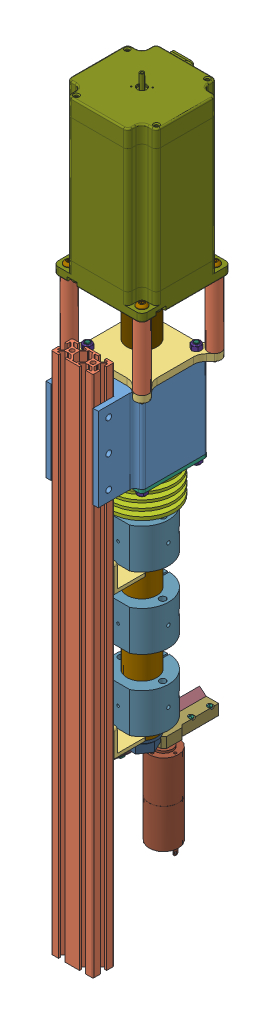
SolidWorks assembly standalone extruder, configuration Default. Lengths in mm.
Overall size (85.21 706.93 142.23).
73 component instances, 27 part files, 167 mates.
Components (placement in the parent):
- hopper rev02-1: hopper rev02 [Default] at (27.6432 17.1739 46.7145) size (63.5 80 98.5)
- 500mm 2040-1: 500mm 2040 [Default] at (27.6432 125.0393 103.4645) x (0 0 1) z (0 1 0) size (20 40 500)
- thrust bearing plate-1: thrust bearing plate [Default] at (27.6432 97.1739 46.7145) size (83.7 6.35 85.2)
- 5909K310_THRUST NEEDLE-ROLLER BEARING-1: 5909K310_THRUST NEEDLE-ROLLER BEARING [5909K31] at (27.6432 95.3689 46.7145) size (23.81 19.84 23.81)
- 5909K440_THRUST NEEDLE-ROLLER BEARING-1: 5909K440_THRUST NEEDLE-ROLLER BEARING [5909K44] at (27.6432 93.5639 46.7145) x (0 1 0) z (0.735724 0 0.677282) size (0.81 23.81 23.81)
- 5909K440_THRUST NEEDLE-ROLLER BEARING-2: 5909K440_THRUST NEEDLE-ROLLER BEARING [5909K44] at (27.6432 96.3611 46.7145) x (0 1 0) z (-0.546944 0 0.837169) size (0.81 23.81 23.81)
- barrel lock mount-1: barrel lock mount [Default] at (27.6432 17.1739 46.7145) x (-1 0 0) z (0 0 1) size (63.5 3.17 63.5)
- barrel lock-1: barrel lock [Default] at (27.6432 -17.7511 46.7145) x (-0.997738 0 -0.067218) z (0.067218 0 -0.997738) size (60.96 31.75 60.96)
- screw standin-1: screw standin [Default] at (27.6432 -173.1361 46.7145) x (0.133635 0 0.991031) z (-0.991031 0 0.133635) size (19.05 324.71 19.05)
- extruder barrel_rev01-1: extruder barrel_rev01 [Default] at (27.6432 93.3739 46.7145) x (1 0 0) z (0 -1 0) size (28.57 28.57 304.8)
- nozzle_rev01-1: nozzle_rev01 [Default] at (27.6432 -192.3761 46.7145) x (0.565776 0 -0.824559) z (0 -1 0) size (28.57 28.57 31.75)
- 3262_1-1: 3262_1 [Default] at (18.029 -323.6244 16.239) x (1 0 0) z (0 1 0) size (28 28 106.2)
- blade wheel-1: blade wheel [Default] at (18.029 -229.4244 16.239) x (0 0 -1) z (-1 0 0) size (90 10 20)
- blade fin-1: blade fin [Default] at (19.9663 -232.1583 46.2387) x (-0.766044 -0.642788 0) z (0 0 -1) size (23.8 0.5 30)
- blade fin-2: blade fin [Default] at (16.0917 -232.1583 -13.7606) x (0.766044 -0.642788 0) z (0 0 1) size (23.8 0.5 30)
- dual cartridge heater block pelletizer-1: dual cartridge heater block pelletizer [Default] at (27.6432 -200.2361 46.7145) x (0 0 1) z (-1 0 0) size (48.25 38.1 50.8)
- dual cartridge heater block pelletizer-2: dual cartridge heater block pelletizer [Default] at (27.6432 -132.1361 46.7145) x (0 0 1) z (-1 0 0) size (48.25 38.1 50.8)
- dual cartridge heater block pelletizer-3: dual cartridge heater block pelletizer [Default] at (27.6432 -64.0361 46.7145) x (0 0 1) z (-1 0 0) size (48.25 38.1 50.8)
- 93325A413_GRADE B7 MEDIUM STRENGTH STEEL THREADED ROD-1: 93325A413_GRADE B7 MEDIUM STRENGTH STEEL THREADED ROD [93325A413] at (53.686 58.9989 20.6718) x (0 -1 0) z (0 0 1) size (101.5 5.07 5.77)
- 93325A413_GRADE B7 MEDIUM STRENGTH STEEL THREADED ROD-2: 93325A413_GRADE B7 MEDIUM STRENGTH STEEL THREADED ROD [93325A413] at (53.686 58.9989 72.7573) x (0 -1 0) z (-0.546944 0 0.837169) size (101.5 5.07 5.77)
- 93325A413_GRADE B7 MEDIUM STRENGTH STEEL THREADED ROD-3: 93325A413_GRADE B7 MEDIUM STRENGTH STEEL THREADED ROD [93325A413] at (1.6005 58.9989 72.7573) x (0 1 0) z (-0.546944 0 0.837169) size (101.5 5.07 5.77)
- 93325A413_GRADE B7 MEDIUM STRENGTH STEEL THREADED ROD-4: 93325A413_GRADE B7 MEDIUM STRENGTH STEEL THREADED ROD [93325A413] at (1.6005 58.9989 20.6718) x (0 -1 0) z (-0.546944 0 0.837169) size (101.5 5.07 5.77)
- nema 34-1: nema 34 [Default] at (27.6432 165.5239 46.7145) x (1 0 0) z (0 -1 0) size (85.21 93.2 198.32)
- 94645A102_ZINC-PLATED CLASS 10 STL NYLON-INSERT LOCKNUT-1: 94645A102_ZINC-PLATED CLASS 10 STL NYLON-INSERT LOCKNUT [94645A102] at (53.686 103.5239 72.7573) size (8 5.15 9.24)
- 94645A102_ZINC-PLATED CLASS 10 STL NYLON-INSERT LOCKNUT-2: 94645A102_ZINC-PLATED CLASS 10 STL NYLON-INSERT LOCKNUT [94645A102] at (53.686 103.5239 20.6718) size (8 5.15 9.24)
- 94645A102_ZINC-PLATED CLASS 10 STL NYLON-INSERT LOCKNUT-3: 94645A102_ZINC-PLATED CLASS 10 STL NYLON-INSERT LOCKNUT [94645A102] at (1.6005 103.5239 72.7573) size (8 5.15 9.24)
- 94645A102_ZINC-PLATED CLASS 10 STL NYLON-INSERT LOCKNUT-4: 94645A102_ZINC-PLATED CLASS 10 STL NYLON-INSERT LOCKNUT [94645A102] at (1.6005 103.5239 20.6718) size (8 5.15 9.24)
- 94645A102_ZINC-PLATED CLASS 10 STL NYLON-INSERT LOCKNUT-5: 94645A102_ZINC-PLATED CLASS 10 STL NYLON-INSERT LOCKNUT [94645A102] at (53.686 13.9989 20.6718) x (-0.5 0 -0.866025) z (-0.866025 0 0.5) size (8 5.15 9.24)
- 94645A102_ZINC-PLATED CLASS 10 STL NYLON-INSERT LOCKNUT-6: 94645A102_ZINC-PLATED CLASS 10 STL NYLON-INSERT LOCKNUT [94645A102] at (53.686 13.9989 72.7573) x (-0.5 0 -0.866025) z (-0.866025 0 0.5) size (8 5.15 9.24)
- 94645A102_ZINC-PLATED CLASS 10 STL NYLON-INSERT LOCKNUT-7: 94645A102_ZINC-PLATED CLASS 10 STL NYLON-INSERT LOCKNUT [94645A102] at (1.6005 13.9989 72.7573) x (-0.5 0 -0.866025) z (-0.866025 0 0.5) size (8 5.15 9.24)
- 94645A102_ZINC-PLATED CLASS 10 STL NYLON-INSERT LOCKNUT-8: 94645A102_ZINC-PLATED CLASS 10 STL NYLON-INSERT LOCKNUT [94645A102] at (1.6005 13.9989 20.6718) x (-0.5 0 -0.866025) z (-0.866025 0 0.5) size (8 5.15 9.24)
- motor coupler-1: motor coupler [Default] at (27.6432 111.6639 46.7145) x (-1 0 0) z (0 0 -1) size (28.57 40 28.57)
- 93245A110_NONMARRING FLAT POINT SOCKET SET SCREW-3: 93245A110_NONMARRING FLAT POINT SOCKET SET SCREW [93245A110] at (27.6432 145.3139 34.7745) x (-0.923728 -0.383049 0) z (0 0 -1) size (4.62 4.16 4.74)
- 93245A110_NONMARRING FLAT POINT SOCKET SET SCREW-4: 93245A110_NONMARRING FLAT POINT SOCKET SET SCREW [93245A110] at (19.2932 118.0139 46.7145) x (0 0.992337 0.12356) z (-1 0 0) size (4.62 4.16 4.74)
- 93245A110_NONMARRING FLAT POINT SOCKET SET SCREW-5: 93245A110_NONMARRING FLAT POINT SOCKET SET SCREW [93245A110] at (27.6432 118.0139 38.3645) x (-0.923728 -0.383049 0) z (0 0 -1) size (4.62 4.16 4.74)
- 93245A110_NONMARRING FLAT POINT SOCKET SET SCREW-6: 93245A110_NONMARRING FLAT POINT SOCKET SET SCREW [93245A110] at (17.7057 145.3139 46.7145) x (0 0.989125 0.14708) z (-1 0 0) size (4.62 4.16 4.74)
- 93245A110_NONMARRING FLAT POINT SOCKET SET SCREW-8: 93245A110_NONMARRING FLAT POINT SOCKET SET SCREW [93245A110] at (28.6332 1.6073 32.0204) x (-0.924173 -0.376865 -0.062262) z (0.067218 0 -0.997738) size (4.62 4.16 4.74)
- motor standoff-1: motor standoff [Default] at (62.3932 103.5239 81.4645) size (12.7 62 12.7)
- motor standoff-2: motor standoff [Default] at (62.3932 103.5239 11.9645) size (12.7 62 12.7)
- motor standoff-3: motor standoff [Default] at (-7.1068 103.5239 81.4645) size (12.7 62 12.7)
- motor standoff-4: motor standoff [Default] at (-7.1068 103.5239 11.9645) size (12.7 62 12.7)
- extruder support-1: extruder support [Default] at (7.6432 -203.4111 93.4645) x (0 -1 0) z (0 0 1) size (25.4 40 31.75)
- extruder support-2: extruder support [Default] at (7.6432 -67.2111 93.4645) x (0 -1 0) z (0 0 1) size (25.4 40 31.75)
- 91239A222_CLASS 10.9 STL BUTTON-HEAD SOCKET CAP SCREW-1: 91239A222_CLASS 10.9 STL BUTTON-HEAD SOCKET CAP SCREW [91239A222] at (17.6432 -206.1611 65.2883) x (1 0 0) z (0 -1 0) size (9.5 9.5 11.19)
- 91239A222_CLASS 10.9 STL BUTTON-HEAD SOCKET CAP SCREW-2: 91239A222_CLASS 10.9 STL BUTTON-HEAD SOCKET CAP SCREW [91239A222] at (37.6432 -206.1611 65.2883) x (1 0 0) z (0 -1 0) size (9.5 9.5 11.19)
- 91239A222_CLASS 10.9 STL BUTTON-HEAD SOCKET CAP SCREW-3: 91239A222_CLASS 10.9 STL BUTTON-HEAD SOCKET CAP SCREW [91239A222] at (37.6432 -69.9611 65.2883) x (1 0 0) z (0 -1 0) size (9.5 9.5 11.19)
- 91239A222_CLASS 10.9 STL BUTTON-HEAD SOCKET CAP SCREW-4: 91239A222_CLASS 10.9 STL BUTTON-HEAD SOCKET CAP SCREW [91239A222] at (17.6432 -69.9611 65.2883) x (1 0 0) z (0 -1 0) size (9.5 9.5 11.19)
- 94180A331_METRIC BRASS HEAT-SET INSERT FOR PLASTICS-1: 94180A331_METRIC BRASS HEAT-SET INSERT FOR PLASTICS [94180A331] at (19.5702 -234.4244 -22.7606) x (-0.492131 0.412947 -0.766344) z (-0.587053 0.492596 0.642431) size (5.56 4.12 5.56)
- 94180A331_METRIC BRASS HEAT-SET INSERT FOR PLASTICS-2: 94180A331_METRIC BRASS HEAT-SET INSERT FOR PLASTICS [94180A331] at (19.5702 -234.4244 -4.7606) x (-0.492131 0.412947 -0.766344) z (-0.587053 0.492596 0.642431) size (5.56 4.12 5.56)
- 94180A331_METRIC BRASS HEAT-SET INSERT FOR PLASTICS-3: 94180A331_METRIC BRASS HEAT-SET INSERT FOR PLASTICS [94180A331] at (16.4877 -234.4244 37.2387) x (-0.613114 -0.514464 -0.599514) z (-0.459255 -0.38536 0.800364) size (5.56 4.12 5.56)
- 94180A331_METRIC BRASS HEAT-SET INSERT FOR PLASTICS-4: 94180A331_METRIC BRASS HEAT-SET INSERT FOR PLASTICS [94180A331] at (16.4877 -234.4244 55.2387) x (-0.613114 -0.514464 -0.599514) z (-0.459255 -0.38536 0.800364) size (5.56 4.12 5.56)
- 92095A181_18-8 SS BUTTON-HEAD SOCKET CAP SCREW-1: 92095A181_18-8 SS BUTTON-HEAD SOCKET CAP SCREW [92095A181] at (17.8697 -236.0714 55.2387) x (0.586824 0.492404 -0.642788) z (0.642788 -0.766044 0) size (5.7 5.7 9.95)
- 92095A181_18-8 SS BUTTON-HEAD SOCKET CAP SCREW-2: 92095A181_18-8 SS BUTTON-HEAD SOCKET CAP SCREW [92095A181] at (17.8697 -236.0714 37.2387) x (0.586824 0.492404 -0.642788) z (0.642788 -0.766044 0) size (5.7 5.7 9.95)
- 92095A181_18-8 SS BUTTON-HEAD SOCKET CAP SCREW-3: 92095A181_18-8 SS BUTTON-HEAD SOCKET CAP SCREW [92095A181] at (18.1882 -236.0714 -4.7606) x (0.586824 -0.492404 0.642788) z (-0.642788 -0.766044 0) size (5.7 5.7 9.95)
- 92095A181_18-8 SS BUTTON-HEAD SOCKET CAP SCREW-4: 92095A181_18-8 SS BUTTON-HEAD SOCKET CAP SCREW [92095A181] at (18.1882 -236.0714 -22.7606) x (0.586824 -0.492404 0.642788) z (-0.642788 -0.766044 0) size (5.7 5.7 9.95)
- 94180A331_METRIC BRASS HEAT-SET INSERT FOR PLASTICS-5: 94180A331_METRIC BRASS HEAT-SET INSERT FOR PLASTICS [94180A331] at (8.029 -234.4244 16.239) x (0 -0.381849 0.924225) z (0 -0.924225 -0.381849) size (5.56 4.12 5.56)
- 92095A181_18-8 SS BUTTON-HEAD SOCKET CAP SCREW-5: 92095A181_18-8 SS BUTTON-HEAD SOCKET CAP SCREW [92095A181] at (5.8682 -234.4244 16.239) x (0 0 1) z (-1 0 0) size (5.7 5.7 9.95)
- 91239A222_CLASS 10.9 STL BUTTON-HEAD SOCKET CAP SCREW-5: 91239A222_CLASS 10.9 STL BUTTON-HEAD SOCKET CAP SCREW [91239A222] at (17.6432 -52.9236 87.5395) x (-0.923728 -0.383049 0) z (0 0 -1) size (9.5 9.5 11.19)
- 91239A222_CLASS 10.9 STL BUTTON-HEAD SOCKET CAP SCREW-6: 91239A222_CLASS 10.9 STL BUTTON-HEAD SOCKET CAP SCREW [91239A222] at (37.6432 -52.9236 87.5395) x (-0.923728 -0.383049 0) z (0 0 -1) size (9.5 9.5 11.19)
- 91239A222_CLASS 10.9 STL BUTTON-HEAD SOCKET CAP SCREW-7: 91239A222_CLASS 10.9 STL BUTTON-HEAD SOCKET CAP SCREW [91239A222] at (37.6432 -189.1236 87.5395) x (-0.923728 -0.383049 0) z (0 0 -1) size (9.5 9.5 11.19)
- 91239A222_CLASS 10.9 STL BUTTON-HEAD SOCKET CAP SCREW-8: 91239A222_CLASS 10.9 STL BUTTON-HEAD SOCKET CAP SCREW [91239A222] at (17.6432 -189.1236 87.5395) x (-0.923728 -0.383049 0) z (0 0 -1) size (9.5 9.5 11.19)
- HNKK5-5-1: HNKK5-5 [Default] at (17.6432 -189.1236 95.4645) x (0 0 -1) z (0 1 0) size (3 10 15)
- HNKK5-5-2: HNKK5-5 [Default] at (37.6432 -189.1236 95.4645) x (0 0 -1) z (0 1 0) size (3 10 15)
- HNKK5-5-3: HNKK5-5 [Default] at (17.6432 -52.9236 95.4645) x (0 0 -1) z (0 1 0) size (3 10 15)
- HNKK5-5-4: HNKK5-5 [Default] at (37.6432 -52.9236 95.4645) x (0 0 -1) z (0 1 0) size (3 10 15)
- 92125A208_TYPE 18-8 SS FLAT-HEAD SOCKET CAP SCREW-1: 92125A208_TYPE 18-8 SS FLAT-HEAD SOCKET CAP SCREW [92125A208] at (13.2748 17.1739 61.0829) x (-0.837169 0 -0.546944) z (0 1 0) size (10 10 10.44)
- 92125A208_TYPE 18-8 SS FLAT-HEAD SOCKET CAP SCREW-2: 92125A208_TYPE 18-8 SS FLAT-HEAD SOCKET CAP SCREW [92125A208] at (13.2748 17.1739 32.3461) x (-0.837169 0 -0.546944) z (0 1 0) size (10 10 10.44)
- 92125A208_TYPE 18-8 SS FLAT-HEAD SOCKET CAP SCREW-3: 92125A208_TYPE 18-8 SS FLAT-HEAD SOCKET CAP SCREW [92125A208] at (42.0116 17.1739 61.0829) x (-0.837169 0 -0.546944) z (0 1 0) size (10 10 10.44)
- 92125A208_TYPE 18-8 SS FLAT-HEAD SOCKET CAP SCREW-4: 92125A208_TYPE 18-8 SS FLAT-HEAD SOCKET CAP SCREW [92125A208] at (42.0116 17.1739 32.3461) x (-0.837169 0 -0.546944) z (0 1 0) size (10 10 10.44)
- 92095A485_18-8 SS BUTTON-HEAD SOCKET CAP SCREW-1: 92095A485_18-8 SS BUTTON-HEAD SOCKET CAP SCREW [92095A485] at (62.3932 176.2739 11.9645) x (1 0 0) z (0 1 0) size (9.5 9.5 83.62)
- 92095A485_18-8 SS BUTTON-HEAD SOCKET CAP SCREW-2: 92095A485_18-8 SS BUTTON-HEAD SOCKET CAP SCREW [92095A485] at (62.3932 176.2739 81.4645) x (1 0 0) z (0 1 0) size (9.5 9.5 83.62)
- 92095A485_18-8 SS BUTTON-HEAD SOCKET CAP SCREW-3: 92095A485_18-8 SS BUTTON-HEAD SOCKET CAP SCREW [92095A485] at (-7.1068 176.2739 81.4645) x (1 0 0) z (0 1 0) size (9.5 9.5 83.62)
- 92095A485_18-8 SS BUTTON-HEAD SOCKET CAP SCREW-4: 92095A485_18-8 SS BUTTON-HEAD SOCKET CAP SCREW [92095A485] at (-7.1068 176.2739 11.9645) x (1 0 0) z (0 1 0) size (9.5 9.5 83.62)
Mates (geometry in assembly coordinates):
- Parallel1: parallel: plane of hopper rev02-1 through (27.6432 17.1739 46.7145) normal (0 -1 0); plane of assembly through (0 0 0) normal (0 1 0)
- Parallel2: parallel: plane of hopper rev02-1 through (-4.1068 97.1739 14.9645) normal (-1 0 0); plane of assembly through (0 0 0) normal (1 0 0)
- Coincident3: coincident anti-aligned: plane of hopper rev02-1 through (47.6432 97.1739 113.4645) normal (-1 0 0); plane of 500mm 2040-1 through (47.6432 -374.9607 100.4645) normal (1 0 0)
- Coincident6: coincident aligned: plane of hopper rev02-1 through (27.6432 97.1739 46.7145) normal (0 1 0); plane of 5909K440_THRUST NEEDLE-ROLLER BEARING-2 through (27.6432 97.1739 46.7145) normal (0 1 0)
- Concentric1: concentric aligned: cylinder of 5909K310_THRUST NEEDLE-ROLLER BEARING-1 through (27.6432 94.3767 46.7145) axis (0 -1 0) radius 11.9062; cylinder of 5909K440_THRUST NEEDLE-ROLLER BEARING-2 through (27.6432 97.1739 46.7145) axis (0 -1 0) radius 11.9062
- Tangent1: tangent anti-aligned: cylinder of 5909K310_THRUST NEEDLE-ROLLER BEARING-1 through (19.3852 95.3689 39.1124) axis (-0.735724 0 -0.677282) radius 0.9922; plane of 5909K440_THRUST NEEDLE-ROLLER BEARING-2 through (27.6432 96.3611 46.7145) normal (0 -1 0)
- Tangent2: tangent anti-aligned: cylinder of 5909K310_THRUST NEEDLE-ROLLER BEARING-1 through (19.3852 95.3689 39.1124) axis (-0.735724 0 -0.677282) radius 0.9922; plane of 5909K440_THRUST NEEDLE-ROLLER BEARING-1 through (27.6432 94.3767 46.7145) normal (0 1 0)
- Concentric2: concentric aligned: circle of 5909K440_THRUST NEEDLE-ROLLER BEARING-1; circle of 5909K440_THRUST NEEDLE-ROLLER BEARING-2
- Concentric3: concentric anti-aligned: cylinder of hopper rev02-1 through (27.6432 17.1729 46.7145) axis (0 1 0) radius 14.2875; cylinder of 5909K440_THRUST NEEDLE-ROLLER BEARING-2 through (27.6432 97.1739 46.7145) axis (0 -1 0) radius 11.9062
- Coincident8: coincident anti-aligned: plane of hopper rev02-1 through (27.6432 97.1739 46.7145) normal (0 1 0); plane of thrust bearing plate-1 through (27.6432 97.1739 46.7145) normal (0 -1 0)
- Coincident11: coincident anti-aligned: plane of hopper rev02-1 through (27.6432 17.1739 46.7145) normal (0 -1 0); plane of barrel lock mount-1 through (27.6432 17.1739 46.7145) normal (0 1 0)
- Coincident12: coincident aligned: plane of hopper rev02-1 through (-4.1068 97.1739 14.9645) normal (-1 0 0); plane of barrel lock mount-1 through (-4.1068 13.9989 78.4645) normal (-1 0 0)
- Coincident13: coincident aligned: plane of hopper rev02-1 through (-4.1068 97.1739 14.9645) normal (0 0 -1); plane of barrel lock mount-1 through (-4.1068 13.9989 14.9645) normal (0 0 -1)
- Coincident14: coincident anti-aligned: plane of barrel lock mount-1 through (27.6432 13.9989 46.7145) normal (0 -1 0); plane of barrel lock-1 through (27.6432 13.9989 46.7145) normal (0 1 0)
- Concentric4: concentric aligned: cylinder of barrel lock mount-1 through (27.6432 17.1749 46.7145) axis (0 -1 0) radius 14.3129; cylinder of barrel lock-1 through (27.6432 13.9989 46.7145) axis (0 -1 0) radius 14.3129
- Concentric5: concentric aligned: cylinder of barrel lock mount-1 through (13.2748 17.1739 32.3461) axis (0 1 0) radius 2.9; cylinder of barrel lock-1 through (13.2748 13.9989 32.3461) axis (0 1 0) radius 2.1
- Concentric6: concentric aligned: cylinder of 5909K440_THRUST NEEDLE-ROLLER BEARING-2 through (27.6432 97.1739 46.7145) axis (0 -1 0) radius 6.3754; cylinder of screw standin-1 through (27.6432 131.6639 46.7145) axis (0 -1 0) radius 6.35
- Coincident15: coincident anti-aligned: plane of 5909K440_THRUST NEEDLE-ROLLER BEARING-1 through (27.6432 93.5639 46.7145) normal (0 -1 0); circle of screw standin-1
- Concentric7: concentric anti-aligned: cylinder of barrel lock-1 through (27.6432 13.9989 46.7145) axis (0 -1 0) radius 14.3129; cylinder of extruder barrel_rev01-1 through (27.6432 -211.4261 46.7145) axis (0 1 0) radius 14.2875
- Coincident16: coincident: line of hopper rev02-1 through (13.3557 17.1739 46.7145) axis (1 0 0); plane of extruder barrel_rev01-1 through (13.3557 17.1739 46.7145) normal (0 0 -1)
- Coincident17: coincident anti-aligned: plane of hopper rev02-1 through (27.6432 17.1739 46.7145) normal (0 -1 0); plane of extruder barrel_rev01-1 through (27.6432 17.1739 46.7145) normal (0 1 0)
- Concentric8: concentric anti-aligned: cylinder of extruder barrel_rev01-1 through (27.6432 -192.3761 46.7145) axis (0 -1 0) radius 11.1125; cylinder of nozzle_rev01-1 through (27.6432 -211.4261 46.7145) axis (0 1 0) radius 11.1125
- Coincident18: coincident anti-aligned: plane of extruder barrel_rev01-1 through (27.6432 -211.4261 46.7145) normal (0 -1 0); plane of nozzle_rev01-1 through (27.6432 -211.4261 46.7145) normal (0 1 0)
- Distance1: distance = 3 mm aligned: plane of 3262_1-1 through (17.8685 -226.4244 16.239) normal (0 1 0); plane of blade wheel-1 through (18.029 -229.4244 16.239) normal (0 1 0)
- Concentric11: concentric aligned: cylinder of 3262_1-1 through (18.029 -243.1244 16.239) axis (0 1 0) radius 3; cylinder of blade wheel-1 through (18.029 -239.4244 16.239) axis (0 1 0) radius 3.165
- Parallel5: parallel aligned: plane of 3262_1-1 through (15.5182 -241.1244 16.239) normal (-1 0 0); plane of blade wheel-1 through (8.029 -201.1402 26.239) normal (-1 0 0)
- Concentric13: concentric aligned: cylinder of blade wheel-1 through (10.5299 -227.3241 55.2387) axis (0.642788 -0.766044 0) radius 2.5; circle of blade fin-1
- Concentric15: concentric anti-aligned: cylinder of blade wheel-1 through (25.5281 -227.3241 -22.7606) axis (-0.642788 -0.766044 0) radius 2.5; cylinder of blade fin-2 through (19.2482 -234.8082 -22.7606) axis (0.642788 0.766044 0) radius 1.665
- Concentric16: concentric anti-aligned: cylinder of extruder barrel_rev01-1 through (27.6432 -211.4261 46.7145) axis (0 1 0) radius 14.2875; cylinder of dual cartridge heater block pelletizer-1 through (27.6432 -162.1361 46.7145) axis (0 -1 0) radius 14.2875
- Distance2: distance = 15 mm aligned: plane of nozzle_rev01-1 through (27.6432 -215.2361 46.7145) normal (0 -1 0); plane of dual cartridge heater block pelletizer-1 through (27.6432 -200.2361 46.7145) normal (0 -1 0)
- Concentric17: concentric anti-aligned: cylinder of extruder barrel_rev01-1 through (27.6432 -211.4261 46.7145) axis (0 1 0) radius 14.2875; cylinder of dual cartridge heater block pelletizer-2 through (27.6432 -94.0361 46.7145) axis (0 -1 0) radius 14.2875
- Coincident38: coincident aligned: plane of dual cartridge heater block pelletizer-1 through (38.7148 -200.2371 69.5745) normal (0 0 1); plane of dual cartridge heater block pelletizer-2 through (38.7148 -132.1371 69.5745) normal (0 0 1)
- Distance3: distance = 30 mm anti-aligned: plane of dual cartridge heater block pelletizer-2 through (27.6432 -132.1361 46.7145) normal (0 -1 0); plane of dual cartridge heater block pelletizer-1 through (27.6432 -162.1361 46.7145) normal (0 1 0)
- Concentric18: concentric anti-aligned: cylinder of extruder barrel_rev01-1 through (27.6432 -211.4261 46.7145) axis (0 1 0) radius 14.2875; cylinder of dual cartridge heater block pelletizer-3 through (27.6432 -25.9361 46.7145) axis (0 -1 0) radius 14.2875
- Coincident40: coincident aligned: plane of dual cartridge heater block pelletizer-2 through (38.7148 -132.1371 69.5745) normal (0 0 1); plane of dual cartridge heater block pelletizer-3 through (38.7148 -64.0371 69.5745) normal (0 0 1)
- Distance4: distance = 30 mm anti-aligned: plane of dual cartridge heater block pelletizer-3 through (27.6432 -64.0361 46.7145) normal (0 -1 0); plane of dual cartridge heater block pelletizer-2 through (27.6432 -94.0361 46.7145) normal (0 1 0)
- Concentric20: concentric anti-aligned: circle of barrel lock mount-1; circle of 93325A413_GRADE B7 MEDIUM STRENGTH STEEL THREADED ROD-1
- Distance5: distance = 5 mm aligned: plane of 93325A413_GRADE B7 MEDIUM STRENGTH STEEL THREADED ROD-1 through (53.686 8.9989 20.6718) normal (0 -1 0); plane of barrel lock mount-1 through (27.6432 13.9989 46.7145) normal (0 -1 0)
- Coincident43: coincident aligned: plane of 93325A413_GRADE B7 MEDIUM STRENGTH STEEL THREADED ROD-1 through (53.686 8.9989 20.6718) normal (0 -1 0); plane of 93325A413_GRADE B7 MEDIUM STRENGTH STEEL THREADED ROD-2 through (53.686 8.9989 72.7573) normal (0 -1 0)
- Concentric21: concentric anti-aligned: cylinder of barrel lock mount-1 through (53.686 13.9979 72.7573) axis (0 1 0) radius 2.6162; circle of 93325A413_GRADE B7 MEDIUM STRENGTH STEEL THREADED ROD-2
- Coincident44: coincident aligned: plane of 93325A413_GRADE B7 MEDIUM STRENGTH STEEL THREADED ROD-1 through (53.686 8.9989 20.6718) normal (0 -1 0); plane of 93325A413_GRADE B7 MEDIUM STRENGTH STEEL THREADED ROD-4 through (1.6005 8.9989 20.6718) normal (0 -1 0)
- Concentric22: concentric anti-aligned: cylinder of barrel lock mount-1 through (1.6005 13.9979 20.6718) axis (0 1 0) radius 2.6162; circle of 93325A413_GRADE B7 MEDIUM STRENGTH STEEL THREADED ROD-4
- Coincident45: coincident aligned: plane of 93325A413_GRADE B7 MEDIUM STRENGTH STEEL THREADED ROD-3 through (1.6005 8.9989 72.7573) normal (0 -1 0); plane of 93325A413_GRADE B7 MEDIUM STRENGTH STEEL THREADED ROD-4 through (1.6005 8.9989 20.6718) normal (0 -1 0)
- Concentric23: concentric anti-aligned: cylinder of barrel lock mount-1 through (1.6005 13.9979 72.7573) axis (0 1 0) radius 2.6162; circle of 93325A413_GRADE B7 MEDIUM STRENGTH STEEL THREADED ROD-3
- Concentric24: concentric anti-aligned: cylinder of screw standin-1 through (27.6432 131.6639 46.7145) axis (0 -1 0) radius 6.35; cylinder of nema 34-1 through (27.6432 80.8533 46.7145) axis (0 1 0) radius 7.9375
- Parallel8: parallel aligned: plane of hopper rev02-1 through (-4.1068 97.1739 14.9645) normal (0 0 -1); plane of nema 34-1 through (52.6432 561.6977 4.1135) normal (0 0 -1)
- Coincident47: coincident anti-aligned: plane of hopper rev02-1 through (27.6432 17.1739 93.4645) normal (0 0 1); plane of 500mm 2040-1 through (34.6432 -374.9607 93.4645) normal (0 0 -1)
- Concentric25: concentric anti-aligned: cylinder of thrust bearing plate-1 through (27.6432 97.1729 46.7145) axis (0 1 0) radius 6.6675; cylinder of screw standin-1 through (27.6432 131.6639 46.7145) axis (0 -1 0) radius 6.35
- Coincident49: coincident anti-aligned: plane of thrust bearing plate-1 through (27.6432 103.5239 46.7145) normal (0 1 0); plane of 94645A102_ZINC-PLATED CLASS 10 STL NYLON-INSERT LOCKNUT-1 through (49.686 103.5239 65.8291) normal (0 -1 0)
- Concentric26: concentric anti-aligned: circle of 93325A413_GRADE B7 MEDIUM STRENGTH STEEL THREADED ROD-2; cylinder of 94645A102_ZINC-PLATED CLASS 10 STL NYLON-INSERT LOCKNUT-1 through (53.686 109.7939 72.7573) axis (0 -1 0) radius 2.6472
- Coincident50: coincident anti-aligned: plane of thrust bearing plate-1 through (27.6432 103.5239 46.7145) normal (0 1 0); plane of 94645A102_ZINC-PLATED CLASS 10 STL NYLON-INSERT LOCKNUT-2 through (49.686 103.5239 13.7436) normal (0 -1 0)
- Concentric27: concentric anti-aligned: circle of 93325A413_GRADE B7 MEDIUM STRENGTH STEEL THREADED ROD-1; cylinder of 94645A102_ZINC-PLATED CLASS 10 STL NYLON-INSERT LOCKNUT-2 through (53.686 109.7939 20.6718) axis (0 -1 0) radius 2.6472
- Coincident51: coincident anti-aligned: plane of thrust bearing plate-1 through (27.6432 103.5239 46.7145) normal (0 1 0); plane of 94645A102_ZINC-PLATED CLASS 10 STL NYLON-INSERT LOCKNUT-3 through (-2.3995 103.5239 65.8291) normal (0 -1 0)
- Concentric28: concentric anti-aligned: circle of 93325A413_GRADE B7 MEDIUM STRENGTH STEEL THREADED ROD-3; cylinder of 94645A102_ZINC-PLATED CLASS 10 STL NYLON-INSERT LOCKNUT-3 through (1.6005 109.7939 72.7573) axis (0 -1 0) radius 2.6472
- Coincident52: coincident anti-aligned: plane of thrust bearing plate-1 through (27.6432 103.5239 46.7145) normal (0 1 0); plane of 94645A102_ZINC-PLATED CLASS 10 STL NYLON-INSERT LOCKNUT-4 through (-2.3995 103.5239 13.7436) normal (0 -1 0)
- Concentric29: concentric anti-aligned: circle of 93325A413_GRADE B7 MEDIUM STRENGTH STEEL THREADED ROD-4; cylinder of 94645A102_ZINC-PLATED CLASS 10 STL NYLON-INSERT LOCKNUT-4 through (1.6005 109.7939 20.6718) axis (0 -1 0) radius 2.6472
- Coincident57: coincident anti-aligned: plane of barrel lock mount-1 through (27.6432 13.9989 46.7145) normal (0 -1 0); plane of 94645A102_ZINC-PLATED CLASS 10 STL NYLON-INSERT LOCKNUT-5 through (61.686 13.9989 20.6718) normal (0 1 0)
- Concentric30: concentric anti-aligned: circle of 93325A413_GRADE B7 MEDIUM STRENGTH STEEL THREADED ROD-1; cylinder of 94645A102_ZINC-PLATED CLASS 10 STL NYLON-INSERT LOCKNUT-5 through (53.686 7.7289 20.6718) axis (0 1 0) radius 2.6472
- Coincident58: coincident anti-aligned: plane of barrel lock mount-1 through (27.6432 13.9989 46.7145) normal (0 -1 0); plane of 94645A102_ZINC-PLATED CLASS 10 STL NYLON-INSERT LOCKNUT-6 through (61.686 13.9989 72.7573) normal (0 1 0)
- Concentric31: concentric anti-aligned: circle of 93325A413_GRADE B7 MEDIUM STRENGTH STEEL THREADED ROD-2; cylinder of 94645A102_ZINC-PLATED CLASS 10 STL NYLON-INSERT LOCKNUT-6 through (53.686 7.7289 72.7573) axis (0 1 0) radius 2.6472
- Coincident59: coincident anti-aligned: plane of barrel lock mount-1 through (27.6432 13.9989 46.7145) normal (0 -1 0); plane of 94645A102_ZINC-PLATED CLASS 10 STL NYLON-INSERT LOCKNUT-7 through (9.6005 13.9989 72.7573) normal (0 1 0)
- Concentric32: concentric anti-aligned: circle of 93325A413_GRADE B7 MEDIUM STRENGTH STEEL THREADED ROD-3; cylinder of 94645A102_ZINC-PLATED CLASS 10 STL NYLON-INSERT LOCKNUT-7 through (1.6005 7.7289 72.7573) axis (0 1 0) radius 2.6472
- Coincident61: coincident anti-aligned: plane of barrel lock mount-1 through (27.6432 13.9989 46.7145) normal (0 -1 0); plane of 94645A102_ZINC-PLATED CLASS 10 STL NYLON-INSERT LOCKNUT-8 through (9.6005 13.9989 20.6718) normal (0 1 0)
- Concentric33: concentric anti-aligned: circle of 93325A413_GRADE B7 MEDIUM STRENGTH STEEL THREADED ROD-4; cylinder of 94645A102_ZINC-PLATED CLASS 10 STL NYLON-INSERT LOCKNUT-8 through (1.6005 7.7289 20.6718) axis (0 1 0) radius 2.6472
- Parallel13: parallel aligned: plane of barrel lock mount-1 through (-4.1068 13.9989 78.4645) normal (-1 0 0); plane of 94645A102_ZINC-PLATED CLASS 10 STL NYLON-INSERT LOCKNUT-7 through (-2.3995 8.9989 75.0667) normal (-1 0 0)
- Parallel14: parallel aligned: plane of barrel lock mount-1 through (-4.1068 13.9989 78.4645) normal (-1 0 0); plane of 94645A102_ZINC-PLATED CLASS 10 STL NYLON-INSERT LOCKNUT-8 through (-2.3995 8.9989 22.9812) normal (-1 0 0)
- Parallel15: parallel aligned: plane of barrel lock mount-1 through (59.3932 13.9989 78.4645) normal (1 0 0); plane of 94645A102_ZINC-PLATED CLASS 10 STL NYLON-INSERT LOCKNUT-5 through (57.686 8.9989 18.3624) normal (1 0 0)
- Parallel16: parallel aligned: plane of barrel lock mount-1 through (59.3932 13.9989 78.4645) normal (1 0 0); plane of 94645A102_ZINC-PLATED CLASS 10 STL NYLON-INSERT LOCKNUT-6 through (57.686 8.9989 70.4479) normal (1 0 0)
- Concentric34: concentric aligned: cylinder of screw standin-1 through (27.6432 131.6639 46.7145) axis (0 -1 0) radius 6.35; cylinder of motor coupler-1 through (27.6432 151.6649 46.7145) axis (0 -1 0) radius 6.3754
- Coincident68: coincident aligned: plane of screw standin-1 through (27.6432 131.6639 46.7145) normal (0 1 0); plane of motor coupler-1 through (27.6432 131.6639 46.7145) normal (0 1 0)
- Parallel17: parallel anti-aligned: plane of nema 34-1 through (30.1432 155.8139 71.8763) normal (1 0 0); plane of motor coupler-1 through (30.2682 125.8567 36.7145) normal (-1 0 0)
- Coincident72: coincident anti-aligned: plane of nema 34-1 through (27.6432 155.8139 36.7745) normal (0 0 -1); plane of 93245A110_NONMARRING FLAT POINT SOCKET SET SCREW-3 through (27.6432 145.3139 36.7745) normal (0 0 1)
- Concentric38: concentric aligned: cylinder of motor coupler-1 through (27.6432 145.3139 32.426) axis (0 0 1) radius 2; circle of 93245A110_NONMARRING FLAT POINT SOCKET SET SCREW-3
- Concentric39: concentric aligned: cylinder of motor coupler-1 through (27.6432 118.0139 32.426) axis (0 0 1) radius 2; circle of 93245A110_NONMARRING FLAT POINT SOCKET SET SCREW-5
- Tangent5: tangent anti-aligned: cylinder of screw standin-1 through (27.6432 131.6639 46.7145) axis (0 -1 0) radius 6.35; plane of 93245A110_NONMARRING FLAT POINT SOCKET SET SCREW-5 through (27.6432 118.0139 40.3645) normal (0 0 1)
- Concentric40: concentric aligned: cylinder of motor coupler-1 through (13.3547 145.3139 46.7145) axis (1 0 0) radius 2; circle of 93245A110_NONMARRING FLAT POINT SOCKET SET SCREW-6
- Tangent6: tangent anti-aligned: cylinder of nema 34-1 through (27.6432 80.8533 46.7145) axis (0 1 0) radius 7.9375; plane of 93245A110_NONMARRING FLAT POINT SOCKET SET SCREW-6 through (19.7057 145.3139 46.7145) normal (1 0 0)
- Concentric41: concentric aligned: cylinder of motor coupler-1 through (13.3547 118.0139 46.7145) axis (1 0 0) radius 2; circle of 93245A110_NONMARRING FLAT POINT SOCKET SET SCREW-4
- Tangent7: tangent anti-aligned: cylinder of screw standin-1 through (27.6432 131.6639 46.7145) axis (0 -1 0) radius 6.35; plane of 93245A110_NONMARRING FLAT POINT SOCKET SET SCREW-4 through (21.2932 118.0139 46.7145) normal (1 0 0)
- Coincident76: coincident anti-aligned: plane of nema 34-1 through (-9.9968 165.5239 84.3545) normal (0 -1 0); plane of motor standoff-1 through (62.3932 165.5239 81.4645) normal (0 1 0)
- Coincident77: coincident anti-aligned: plane of thrust bearing plate-1 through (27.6432 103.5239 46.7145) normal (0 1 0); plane of motor standoff-1 through (62.3932 103.5239 81.4645) normal (0 -1 0)
- Concentric43: concentric aligned: cylinder of nema 34-1 through (62.3932 173.5239 81.4645) axis (0 -1 0) radius 2.875; cylinder of motor standoff-1 through (62.3932 165.5239 81.4645) axis (0 -1 0) radius 2.665
- Coincident78: coincident anti-aligned: plane of nema 34-1 through (-9.9968 165.5239 84.3545) normal (0 -1 0); plane of motor standoff-2 through (62.3932 165.5239 11.9645) normal (0 1 0)
- Concentric44: concentric aligned: cylinder of motor standoff-2 through (62.3932 165.5239 11.9645) axis (0 -1 0) radius 2.665; cylinder of nema 34-1 through (62.3932 173.5239 11.9645) axis (0 -1 0) radius 2.875
- Coincident79: coincident anti-aligned: plane of nema 34-1 through (-9.9968 165.5239 84.3545) normal (0 -1 0); plane of motor standoff-4 through (-7.1068 165.5239 11.9645) normal (0 1 0)
- Concentric45: concentric aligned: cylinder of nema 34-1 through (-7.1068 173.5239 11.9645) axis (0 -1 0) radius 2.875; cylinder of motor standoff-4 through (-7.1068 165.5239 11.9645) axis (0 -1 0) radius 2.665
- Coincident80: coincident anti-aligned: plane of nema 34-1 through (-9.9968 165.5239 84.3545) normal (0 -1 0); plane of motor standoff-3 through (-7.1068 165.5239 81.4645) normal (0 1 0)
- Concentric46: concentric aligned: cylinder of nema 34-1 through (-7.1068 173.5239 81.4645) axis (0 -1 0) radius 2.875; cylinder of motor standoff-3 through (-7.1068 165.5239 81.4645) axis (0 -1 0) radius 2.665
- Coincident81: coincident anti-aligned: plane of 500mm 2040-1 through (34.6432 -374.9607 93.4645) normal (0 0 -1); plane of extruder support-1 through (47.6432 -203.4111 93.4645) normal (0 0 1)
- Coincident82: coincident aligned: plane of 500mm 2040-1 through (7.6432 -374.9607 94.4645) normal (-1 0 0); plane of extruder support-1 through (7.6432 -203.4111 93.4645) normal (-1 0 0)
- Parallel19: parallel anti-aligned: plane of 500mm 2040-1 through (34.6432 -374.9607 93.4645) normal (0 0 -1); plane of dual cartridge heater block pelletizer-1 through (38.7148 -200.2371 69.5745) normal (0 0 1)
- Coincident86: coincident anti-aligned: plane of dual cartridge heater block pelletizer-3 through (27.6432 -64.0361 46.7145) normal (0 -1 0); plane of extruder support-2 through (47.6432 -64.0361 90.2895) normal (0 1 0)
- Concentric47: concentric aligned: cylinder of dual cartridge heater block pelletizer-3 through (17.6432 -54.0361 65.2883) axis (0 -1 0) radius 2.665; cylinder of extruder support-2 through (17.6432 -41.8101 65.2883) axis (0 -1 0) radius 2.665
- Coincident87: coincident aligned: plane of 500mm 2040-1 through (7.6432 -374.9607 94.4645) normal (-1 0 0); plane of extruder support-2 through (7.6432 -67.2111 93.4645) normal (-1 0 0)
- Parallel23: parallel aligned: plane of 500mm 2040-1 through (47.6432 -374.9607 100.4645) normal (1 0 0); plane of blade wheel-1 through (28.029 -201.1402 26.239) normal (1 0 0)
- Coincident106: coincident anti-aligned: plane of blade wheel-1 through (25.529 -239.4244 6.239) normal (-0.642788 -0.766044 0); plane of blade fin-2 through (16.413 -231.7752 -13.7606) normal (0.642788 0.766044 0)
- Concentric64: concentric anti-aligned: cylinder of blade wheel-1 through (25.5281 -227.3241 -4.7606) axis (-0.642788 -0.766044 0) radius 2.5; cylinder of blade fin-2 through (19.2482 -234.8082 -4.7606) axis (0.642788 0.766044 0) radius 1.665
- Concentric65: concentric anti-aligned: cylinder of blade wheel-1 through (25.5281 -227.3241 -22.7606) axis (-0.642788 -0.766044 0) radius 2.5; cylinder of blade fin-2 through (19.2482 -234.8082 -22.7606) axis (0.642788 0.766044 0) radius 1.665
- Coincident107: coincident anti-aligned: plane of blade wheel-1 through (10.529 -239.4244 26.239) normal (0.642788 -0.766044 0); plane of blade fin-1 through (19.6449 -231.7752 46.2387) normal (-0.642788 0.766044 0)
- Concentric66: concentric anti-aligned: cylinder of blade wheel-1 through (10.5299 -227.3241 37.2387) axis (0.642788 -0.766044 0) radius 2.5; cylinder of blade fin-1 through (16.8098 -234.8082 37.2387) axis (-0.642788 0.766044 0) radius 1.665
- Concentric67: concentric anti-aligned: cylinder of blade wheel-1 through (10.5299 -227.3241 55.2387) axis (0.642788 -0.766044 0) radius 2.5; cylinder of blade fin-1 through (16.8098 -234.8082 55.2387) axis (-0.642788 0.766044 0) radius 1.665
- Coincident108: coincident anti-aligned: plane of extruder support-1 through (47.6432 -203.4111 61.7145) normal (0 -1 0); plane of 91239A222_CLASS 10.9 STL BUTTON-HEAD SOCKET CAP SCREW-1 through (17.6432 -203.4111 60.5383) normal (0 1 0)
- Concentric68: concentric aligned: cylinder of extruder support-1 through (17.6432 -178.0101 65.2883) axis (0 -1 0) radius 2.665; cylinder of 91239A222_CLASS 10.9 STL BUTTON-HEAD SOCKET CAP SCREW-1 through (17.6432 -206.1611 65.2883) axis (0 -1 0) radius 4.75
- Coincident109: coincident anti-aligned: plane of extruder support-1 through (47.6432 -203.4111 61.7145) normal (0 -1 0); plane of 91239A222_CLASS 10.9 STL BUTTON-HEAD SOCKET CAP SCREW-2 through (37.6432 -203.4111 60.5383) normal (0 1 0)
- Concentric69: concentric aligned: cylinder of extruder support-1 through (37.6432 -178.0101 65.2883) axis (0 -1 0) radius 2.665; cylinder of 91239A222_CLASS 10.9 STL BUTTON-HEAD SOCKET CAP SCREW-2 through (37.6432 -206.1611 65.2883) axis (0 -1 0) radius 4.75
- Coincident110: coincident anti-aligned: plane of extruder support-2 through (47.6432 -67.2111 61.7145) normal (0 -1 0); plane of 91239A222_CLASS 10.9 STL BUTTON-HEAD SOCKET CAP SCREW-4 through (17.6432 -67.2111 60.5383) normal (0 1 0)
- Concentric70: concentric aligned: cylinder of extruder support-2 through (17.6432 -41.8101 65.2883) axis (0 -1 0) radius 2.665; cylinder of 91239A222_CLASS 10.9 STL BUTTON-HEAD SOCKET CAP SCREW-4 through (17.6432 -69.9611 65.2883) axis (0 -1 0) radius 4.75
- Coincident111: coincident anti-aligned: plane of extruder support-2 through (47.6432 -67.2111 61.7145) normal (0 -1 0); plane of 91239A222_CLASS 10.9 STL BUTTON-HEAD SOCKET CAP SCREW-3 through (37.6432 -67.2111 60.5383) normal (0 1 0)
- Concentric71: concentric aligned: cylinder of extruder support-2 through (37.6432 -41.8101 65.2883) axis (0 -1 0) radius 2.665; cylinder of 91239A222_CLASS 10.9 STL BUTTON-HEAD SOCKET CAP SCREW-3 through (37.6432 -69.9611 65.2883) axis (0 -1 0) radius 4.75
- Coincident112: coincident: plane of nozzle_rev01-1 through (27.6432 -224.1261 46.7145) normal (0 -1 0); line of blade fin-1 through (28.7608 -224.1261 61.2387) axis (0 0 -1)
- Concentric72: concentric aligned: cylinder of blade wheel-1 through (25.5281 -227.3241 -22.7606) axis (-0.642788 -0.766044 0) radius 2.5; cylinder of 94180A331_METRIC BRASS HEAT-SET INSERT FOR PLASTICS-1 through (19.5702 -234.4244 -22.7606) axis (-0.642788 -0.766044 0) radius 2.525
- Coincident113: coincident anti-aligned: plane of blade fin-2 through (16.413 -231.7752 -13.7606) normal (0.642788 0.766044 0); plane of 94180A331_METRIC BRASS HEAT-SET INSERT FOR PLASTICS-1 through (19.5702 -234.4244 -22.7606) normal (-0.642788 -0.766044 0)
- Concentric73: concentric aligned: cylinder of blade wheel-1 through (25.5281 -227.3241 -4.7606) axis (-0.642788 -0.766044 0) radius 2.5; cylinder of 94180A331_METRIC BRASS HEAT-SET INSERT FOR PLASTICS-2 through (19.5702 -234.4244 -4.7606) axis (-0.642788 -0.766044 0) radius 2.525
- Coincident114: coincident anti-aligned: plane of blade fin-2 through (16.413 -231.7752 -13.7606) normal (0.642788 0.766044 0); plane of 94180A331_METRIC BRASS HEAT-SET INSERT FOR PLASTICS-2 through (19.5702 -234.4244 -4.7606) normal (-0.642788 -0.766044 0)
- Concentric74: concentric aligned: cylinder of blade wheel-1 through (10.5299 -227.3241 55.2387) axis (0.642788 -0.766044 0) radius 2.5; cylinder of 94180A331_METRIC BRASS HEAT-SET INSERT FOR PLASTICS-4 through (16.4877 -234.4244 55.2387) axis (0.642788 -0.766044 0) radius 2.525
- Coincident115: coincident anti-aligned: plane of blade fin-1 through (19.6449 -231.7752 46.2387) normal (-0.642788 0.766044 0); plane of 94180A331_METRIC BRASS HEAT-SET INSERT FOR PLASTICS-4 through (16.4877 -234.4244 55.2387) normal (0.642788 -0.766044 0)
- Concentric75: concentric aligned: cylinder of blade wheel-1 through (10.5299 -227.3241 37.2387) axis (0.642788 -0.766044 0) radius 2.5; cylinder of 94180A331_METRIC BRASS HEAT-SET INSERT FOR PLASTICS-3 through (16.4877 -234.4244 37.2387) axis (0.642788 -0.766044 0) radius 2.525
- Coincident116: coincident anti-aligned: plane of blade fin-1 through (19.6449 -231.7752 46.2387) normal (-0.642788 0.766044 0); plane of 94180A331_METRIC BRASS HEAT-SET INSERT FOR PLASTICS-3 through (16.4877 -234.4244 37.2387) normal (0.642788 -0.766044 0)
- Coincident118: coincident anti-aligned: plane of blade fin-1 through (19.9663 -232.1583 46.2387) normal (0.642788 -0.766044 0); plane of 92095A181_18-8 SS BUTTON-HEAD SOCKET CAP SCREW-1 through (15.4058 -235.985 53.0555) normal (-0.642788 0.766044 0)
- Concentric76: concentric anti-aligned: cylinder of blade fin-1 through (16.8098 -234.8082 55.2387) axis (-0.642788 0.766044 0) radius 1.665; cylinder of 92095A181_18-8 SS BUTTON-HEAD SOCKET CAP SCREW-1 through (17.8697 -236.0714 55.2387) axis (0.642788 -0.766044 0) radius 2.85
- Coincident119: coincident anti-aligned: plane of blade fin-1 through (19.9663 -232.1583 46.2387) normal (0.642788 -0.766044 0); plane of 92095A181_18-8 SS BUTTON-HEAD SOCKET CAP SCREW-2 through (15.4058 -235.985 35.0555) normal (-0.642788 0.766044 0)
- Concentric77: concentric anti-aligned: cylinder of blade fin-1 through (16.8098 -234.8082 37.2387) axis (-0.642788 0.766044 0) radius 1.665; cylinder of 92095A181_18-8 SS BUTTON-HEAD SOCKET CAP SCREW-2 through (17.8697 -236.0714 37.2387) axis (0.642788 -0.766044 0) radius 2.85
- Coincident120: coincident anti-aligned: plane of blade fin-2 through (16.0917 -232.1583 -13.7606) normal (-0.642788 -0.766044 0); plane of 92095A181_18-8 SS BUTTON-HEAD SOCKET CAP SCREW-3 through (20.6522 -235.985 -6.9439) normal (0.642788 0.766044 0)
- Concentric78: concentric anti-aligned: cylinder of blade fin-2 through (19.2482 -234.8082 -4.7606) axis (0.642788 0.766044 0) radius 1.665; cylinder of 92095A181_18-8 SS BUTTON-HEAD SOCKET CAP SCREW-3 through (18.1882 -236.0714 -4.7606) axis (-0.642788 -0.766044 0) radius 2.85
- Coincident121: coincident anti-aligned: plane of blade fin-2 through (16.0917 -232.1583 -13.7606) normal (-0.642788 -0.766044 0); plane of 92095A181_18-8 SS BUTTON-HEAD SOCKET CAP SCREW-4 through (20.6522 -235.985 -24.9439) normal (0.642788 0.766044 0)
- Concentric79: concentric anti-aligned: cylinder of blade fin-2 through (19.2482 -234.8082 -22.7606) axis (0.642788 0.766044 0) radius 1.665; cylinder of 92095A181_18-8 SS BUTTON-HEAD SOCKET CAP SCREW-4 through (18.1882 -236.0714 -22.7606) axis (-0.642788 -0.766044 0) radius 2.85
- Concentric80: concentric aligned: cylinder of blade wheel-1 through (28.03 -234.4244 16.239) axis (-1 0 0) radius 2.5; cylinder of 94180A331_METRIC BRASS HEAT-SET INSERT FOR PLASTICS-5 through (8.029 -234.4244 16.239) axis (-1 0 0) radius 2.525
- Coincident122: coincident aligned: plane of blade wheel-1 through (8.029 -201.1402 26.239) normal (-1 0 0); plane of 94180A331_METRIC BRASS HEAT-SET INSERT FOR PLASTICS-5 through (8.029 -234.4244 16.239) normal (-1 0 0)
- Coincident123: coincident anti-aligned: plane of 3262_1-1 through (15.5182 -241.1244 16.239) normal (-1 0 0); plane of 92095A181_18-8 SS BUTTON-HEAD SOCKET CAP SCREW-5 through (15.5182 -235.9244 16.239) normal (1 0 0)
- Concentric81: concentric aligned: cylinder of blade wheel-1 through (28.03 -234.4244 16.239) axis (-1 0 0) radius 2.5; cylinder of 92095A181_18-8 SS BUTTON-HEAD SOCKET CAP SCREW-5 through (5.8682 -234.4244 16.239) axis (-1 0 0) radius 2.85
- Coincident124: coincident anti-aligned: plane of extruder support-2 through (47.6432 -41.8111 90.2895) normal (0 0 -1); plane of 91239A222_CLASS 10.9 STL BUTTON-HEAD SOCKET CAP SCREW-5 through (19.4627 -57.3113 90.2895) normal (0 0 1)
- Concentric82: concentric aligned: cylinder of extruder support-2 through (17.6432 -52.9236 93.4655) axis (0 0 -1) radius 2.665; cylinder of 91239A222_CLASS 10.9 STL BUTTON-HEAD SOCKET CAP SCREW-5 through (17.6432 -52.9236 87.5395) axis (0 0 -1) radius 4.75
- Coincident125: coincident anti-aligned: plane of extruder support-2 through (47.6432 -41.8111 90.2895) normal (0 0 -1); plane of 91239A222_CLASS 10.9 STL BUTTON-HEAD SOCKET CAP SCREW-6 through (39.4627 -57.3113 90.2895) normal (0 0 1)
- Concentric83: concentric aligned: cylinder of extruder support-2 through (37.6432 -52.9236 93.4655) axis (0 0 -1) radius 2.665; cylinder of 91239A222_CLASS 10.9 STL BUTTON-HEAD SOCKET CAP SCREW-6 through (37.6432 -52.9236 87.5395) axis (0 0 -1) radius 4.75
- Coincident126: coincident anti-aligned: plane of extruder support-1 through (47.6432 -178.0111 90.2895) normal (0 0 -1); plane of 91239A222_CLASS 10.9 STL BUTTON-HEAD SOCKET CAP SCREW-8 through (19.4627 -193.5113 90.2895) normal (0 0 1)
- Concentric84: concentric aligned: cylinder of extruder support-1 through (17.6432 -189.1236 93.4655) axis (0 0 -1) radius 2.665; cylinder of 91239A222_CLASS 10.9 STL BUTTON-HEAD SOCKET CAP SCREW-8 through (17.6432 -189.1236 87.5395) axis (0 0 -1) radius 4.75
- Coincident127: coincident anti-aligned: plane of extruder support-1 through (47.6432 -178.0111 90.2895) normal (0 0 -1); plane of 91239A222_CLASS 10.9 STL BUTTON-HEAD SOCKET CAP SCREW-7 through (39.4627 -193.5113 90.2895) normal (0 0 1)
- Concentric85: concentric aligned: cylinder of extruder support-1 through (37.6432 -189.1236 93.4655) axis (0 0 -1) radius 2.665; cylinder of 91239A222_CLASS 10.9 STL BUTTON-HEAD SOCKET CAP SCREW-7 through (37.6432 -189.1236 87.5395) axis (0 0 -1) radius 4.75
- Coincident129: coincident anti-aligned: plane of 500mm 2040-1 through (11.6432 -374.9607 95.4645) normal (0 0 1); plane of HNKK5-5-1 through (21.8932 -182.3736 95.4645) normal (0 0 -1)
- Parallel26: parallel anti-aligned: plane of 500mm 2040-1 through (7.6432 -374.9607 94.4645) normal (-1 0 0); plane of HNKK5-5-1 through (22.6432 -182.3736 98.4645) normal (1 0 0)
- Concentric87: concentric anti-aligned: cylinder of 91239A222_CLASS 10.9 STL BUTTON-HEAD SOCKET CAP SCREW-8 through (17.6432 -189.1236 87.5395) axis (0 0 -1) radius 4.75; cylinder of HNKK5-5-1 through (17.6432 -189.1236 95.4645) axis (0 0 1) radius 2.067
- Coincident132: coincident anti-aligned: plane of 500mm 2040-1 through (40.6432 -374.9607 95.4645) normal (0 0 1); plane of HNKK5-5-2 through (41.8932 -182.3736 95.4645) normal (0 0 -1)
- Parallel27: parallel anti-aligned: plane of 500mm 2040-1 through (7.6432 -374.9607 94.4645) normal (-1 0 0); plane of HNKK5-5-2 through (42.6432 -182.3736 98.4645) normal (1 0 0)
- Concentric88: concentric anti-aligned: cylinder of 91239A222_CLASS 10.9 STL BUTTON-HEAD SOCKET CAP SCREW-7 through (37.6432 -189.1236 87.5395) axis (0 0 -1) radius 4.75; cylinder of HNKK5-5-2 through (37.6432 -189.1236 95.4645) axis (0 0 1) radius 2.067
- Coincident134: coincident anti-aligned: plane of 500mm 2040-1 through (11.6432 -374.9607 95.4645) normal (0 0 1); plane of HNKK5-5-3 through (21.8932 -46.1736 95.4645) normal (0 0 -1)
- Parallel28: parallel anti-aligned: plane of 500mm 2040-1 through (7.6432 -374.9607 94.4645) normal (-1 0 0); plane of HNKK5-5-3 through (22.6432 -46.1736 98.4645) normal (1 0 0)
- Concentric89: concentric anti-aligned: cylinder of 91239A222_CLASS 10.9 STL BUTTON-HEAD SOCKET CAP SCREW-5 through (17.6432 -52.9236 87.5395) axis (0 0 -1) radius 4.75; cylinder of HNKK5-5-3 through (17.6432 -52.9236 95.4645) axis (0 0 1) radius 2.067
- Coincident136: coincident anti-aligned: plane of 500mm 2040-1 through (20.6432 -374.9607 95.4645) normal (0 0 1); plane of HNKK5-5-4 through (41.8932 -46.1736 95.4645) normal (0 0 -1)
- Parallel29: parallel anti-aligned: plane of 500mm 2040-1 through (7.6432 -374.9607 94.4645) normal (-1 0 0); plane of HNKK5-5-4 through (42.6432 -46.1736 98.4645) normal (1 0 0)
- Concentric90: concentric anti-aligned: cylinder of 91239A222_CLASS 10.9 STL BUTTON-HEAD SOCKET CAP SCREW-6 through (37.6432 -52.9236 87.5395) axis (0 0 -1) radius 4.75; cylinder of HNKK5-5-4 through (37.6432 -52.9236 95.4645) axis (0 0 1) radius 2.067
- Concentric91: concentric aligned: cylinder of barrel lock-1 through (29.6921 1.6073 16.3025) axis (-0.067218 0 0.997738) radius 2; circle of 93245A110_NONMARRING FLAT POINT SOCKET SET SCREW-8
- Coincident141: coincident: plane of barrel lock mount-1 through (27.6432 17.1739 46.7145) normal (0 1 0); plane of 92125A208_TYPE 18-8 SS FLAT-HEAD SOCKET CAP SCREW-1 through (14.6422 17.1739 58.99) normal (0 1 0)
- Concentric92: concentric aligned: cylinder of barrel lock mount-1 through (13.2748 17.1739 61.0829) axis (0 1 0) radius 2.9; cylinder of 92125A208_TYPE 18-8 SS FLAT-HEAD SOCKET CAP SCREW-1 through (13.2748 17.1739 61.0829) axis (0 1 0) radius 5
- Coincident142: coincident: plane of barrel lock mount-1 through (27.6432 17.1739 46.7145) normal (0 1 0); plane of 92125A208_TYPE 18-8 SS FLAT-HEAD SOCKET CAP SCREW-2 through (14.6422 17.1739 30.2532) normal (0 1 0)
- Concentric93: concentric aligned: cylinder of barrel lock mount-1 through (13.2748 17.1739 32.3461) axis (0 1 0) radius 2.9; cylinder of 92125A208_TYPE 18-8 SS FLAT-HEAD SOCKET CAP SCREW-2 through (13.2748 17.1739 32.3461) axis (0 1 0) radius 5
- Coincident143: coincident: plane of barrel lock mount-1 through (27.6432 17.1739 46.7145) normal (0 1 0); plane of 92125A208_TYPE 18-8 SS FLAT-HEAD SOCKET CAP SCREW-4 through (43.379 17.1739 30.2532) normal (0 1 0)
- Concentric94: concentric aligned: cylinder of barrel lock mount-1 through (42.0116 17.1739 32.3461) axis (0 1 0) radius 2.9; cylinder of 92125A208_TYPE 18-8 SS FLAT-HEAD SOCKET CAP SCREW-4 through (42.0116 17.1739 32.3461) axis (0 1 0) radius 5
- Coincident144: coincident: plane of barrel lock mount-1 through (27.6432 17.1739 46.7145) normal (0 1 0); plane of 92125A208_TYPE 18-8 SS FLAT-HEAD SOCKET CAP SCREW-3 through (43.379 17.1739 58.99) normal (0 1 0)
- Concentric95: concentric aligned: cylinder of barrel lock mount-1 through (42.0116 17.1739 61.0829) axis (0 1 0) radius 2.9; cylinder of 92125A208_TYPE 18-8 SS FLAT-HEAD SOCKET CAP SCREW-3 through (42.0116 17.1739 61.0829) axis (0 1 0) radius 5
- Coincident145: coincident: plane of nema 34-1 through (-9.9968 173.5239 84.3545) normal (0 1 0); plane of 92095A485_18-8 SS BUTTON-HEAD SOCKET CAP SCREW-1 through (62.3932 173.5239 16.7145) normal (0 -1 0)
- Concentric96: concentric anti-aligned: cylinder of nema 34-1 through (62.3932 173.5239 11.9645) axis (0 -1 0) radius 2.875; cylinder of 92095A485_18-8 SS BUTTON-HEAD SOCKET CAP SCREW-1 through (62.3932 176.2739 11.9645) axis (0 1 0) radius 4.75
- Coincident146: coincident: plane of nema 34-1 through (-9.9968 173.5239 84.3545) normal (0 1 0); plane of 92095A485_18-8 SS BUTTON-HEAD SOCKET CAP SCREW-2 through (62.3932 173.5239 86.2145) normal (0 -1 0)
- Concentric97: concentric anti-aligned: cylinder of nema 34-1 through (62.3932 173.5239 81.4645) axis (0 -1 0) radius 2.875; cylinder of 92095A485_18-8 SS BUTTON-HEAD SOCKET CAP SCREW-2 through (62.3932 176.2739 81.4645) axis (0 1 0) radius 4.75
- Coincident147: coincident: plane of nema 34-1 through (-9.9968 173.5239 84.3545) normal (0 1 0); plane of 92095A485_18-8 SS BUTTON-HEAD SOCKET CAP SCREW-4 through (-7.1068 173.5239 16.7145) normal (0 -1 0)
- Concentric98: concentric anti-aligned: cylinder of nema 34-1 through (-7.1068 173.5239 11.9645) axis (0 -1 0) radius 2.875; cylinder of 92095A485_18-8 SS BUTTON-HEAD SOCKET CAP SCREW-4 through (-7.1068 176.2739 11.9645) axis (0 1 0) radius 4.75
- Coincident148: coincident: plane of nema 34-1 through (-9.9968 173.5239 84.3545) normal (0 1 0); plane of 92095A485_18-8 SS BUTTON-HEAD SOCKET CAP SCREW-3 through (-7.1068 173.5239 86.2145) normal (0 -1 0)
- Concentric99: concentric anti-aligned: cylinder of nema 34-1 through (-7.1068 173.5239 81.4645) axis (0 -1 0) radius 2.875; cylinder of 92095A485_18-8 SS BUTTON-HEAD SOCKET CAP SCREW-3 through (-7.1068 176.2739 81.4645) axis (0 1 0) radius 4.75
